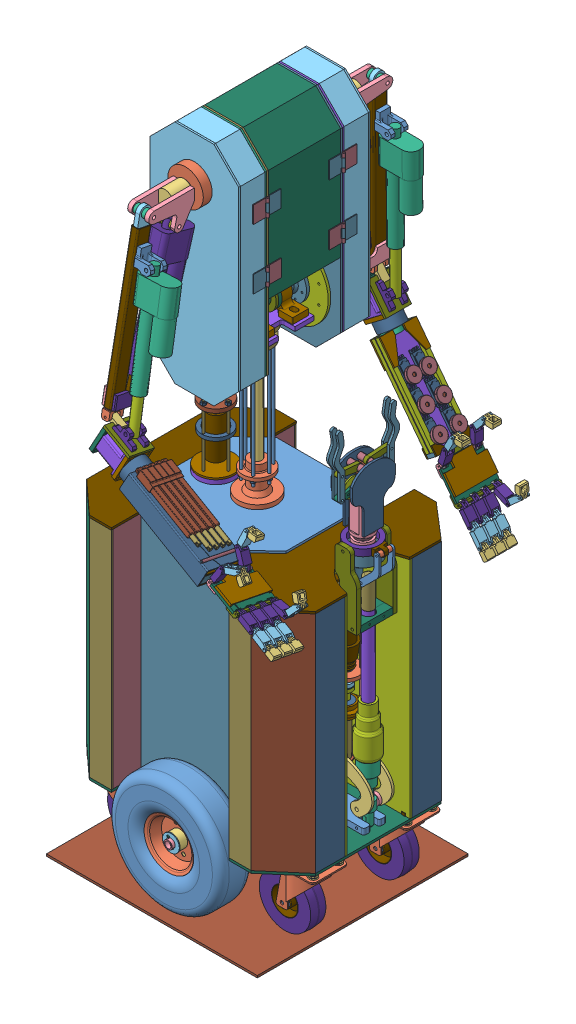
SolidWorks assembly sorbot, configuration По умолчанию. Lengths in mm. (continued)
Mates (geometry in assembly coordinates): (continued)
- Заблокировать432: lock: unknown of ?; unknown of ?
- Заблокировать433: lock: unknown of ?; unknown of ?
- Заблокировать434: lock: unknown of ?; unknown of ?
- Концентричный501: concentric aligned: cylinder of forearm.rotate-2/SY57STH56-2804A-1 through (17.8304 847.8969 -413.8911) axis (-0.604887 0.796311 0.000678) radius 3.175; cylinder of forearm.rotate.p2-2 through (17.165 848.7728 -413.8904) axis (-0.604887 0.796311 0.000678) radius 3.175
- Расстояние24: distance = 2 mm aligned: plane of forearm.rotate-2/forearm.rotate.p4-1 through (24.1212 839.6153 -413.8982) normal (0.604887 -0.796311 -0.000678); plane of forearm.rotate.p2-2 through (25.331 838.0226 -413.8995) normal (0.604887 -0.796311 -0.000678)
- Совпадение891: coincident anti-aligned: plane of forearm.rotate.p2-2 through (25.331 838.0226 -413.8995) normal (0.604887 -0.796311 -0.000678); plane of lower.arm.p1-2 through (36.5459 846.5524 -426.6459) normal (-0.604887 0.796311 0.000678)
- Заблокировать435: lock: unknown of ?; unknown of ?
- Заблокировать436: lock: unknown of ?; unknown of ?
- Заблокировать437: lock: unknown of ?; unknown of ?
- Заблокировать438: lock: unknown of ?; unknown of ?
- Заблокировать439: lock: unknown of ?; unknown of ?
- Заблокировать440: lock: unknown of ?; unknown of ?
- Заблокировать441: lock: unknown of ?; unknown of ?
- Заблокировать442: lock: unknown of ?; unknown of ?
- Заблокировать443: lock: unknown of ?; unknown of ?
- Заблокировать444: lock: unknown of ?; unknown of ?
- Заблокировать445: lock: unknown of ?; unknown of ?
- Параллельность201: parallel aligned: plane of forearm.rotate.p7-2 through (39.1177 879.8642 -383.6264) normal (0.796294 0.604869 0.00704); plane of lower.arm.p3-2 through (25.9039 838.4212 -370.8936) normal (0.796294 0.604869 0.00704)
- Заблокировать446: lock: unknown of ?; unknown of ?
- Заблокировать447: lock: unknown of ?; unknown of ?
- Заблокировать448: lock: unknown of ?; unknown of ?
- Заблокировать449: lock: unknown of ?; unknown of ?
- Заблокировать450: lock: unknown of ?; unknown of ?
- Заблокировать451: lock: unknown of ?; unknown of ?
- Концентричный504: concentric anti-aligned: cylinder of HS-311 Hitec Standard Servo and Horn-12/HS-311-p2-1 through (86.8297 780.9654 -431.4942) axis (0.796294 0.604869 0.00704) radius 4.064; cylinder of lower.arm.p9-8 through (91.8065 784.7458 -431.4502) axis (-0.796294 -0.604869 -0.00704) radius 12
- Концентричный505: concentric anti-aligned: cylinder of HS-311 Hitec Standard Servo and Horn-8/HS-311-p2-1 through (120.1178 737.1736 -434.1714) axis (0.796294 0.604869 0.00704) radius 4.064; cylinder of lower.arm.p9-10 through (125.0946 740.954 -434.1274) axis (-0.796294 -0.604869 -0.00704) radius 12
- Концентричный506: concentric anti-aligned: cylinder of HS-311 Hitec Standard Servo and Horn-10/HS-311-p2-1 through (153.4054 693.3815 -436.7686) axis (0.796294 0.604869 0.00704) radius 4.064; cylinder of lower.arm.p9-12 through (158.3823 697.1619 -436.7246) axis (-0.796294 -0.604869 -0.00704) radius 12
- Концентричный507: concentric anti-aligned: cylinder of HS-311 Hitec Standard Servo and Horn-11/HS-311-p2-1 through (86.6463 780.7961 -396.215) axis (0.796294 0.604869 0.00704) radius 4.064; cylinder of lower.arm.p9-7 through (91.6232 784.5765 -396.171) axis (-0.796294 -0.604869 -0.00704) radius 12
- Концентричный508: concentric anti-aligned: cylinder of HS-311 Hitec Standard Servo and Horn-7/HS-311-p2-1 through (119.907 736.979 -393.6124) axis (0.796294 0.604869 0.00704) radius 4.064; cylinder of lower.arm.p9-9 through (124.8838 740.7594 -393.5684) axis (-0.796294 -0.604869 -0.00704) radius 12
- Концентричный509: concentric anti-aligned: cylinder of HS-311 Hitec Standard Servo and Horn-9/HS-311-p2-1 through (153.1681 693.1623 -391.0897) axis (0.796294 0.604869 0.00704) radius 4.064; cylinder of lower.arm.p9-11 through (158.1449 696.9427 -391.0457) axis (-0.796294 -0.604869 -0.00704) radius 12
- Совпадение938: coincident anti-aligned: plane of HS-311 Hitec Standard Servo and Horn-12/HS-311-p2-1 through (93.1733 783.0442 -439.8505) normal (0.796294 0.604869 0.00704); plane of lower.arm.p9-8 through (91.8065 784.7458 -431.4502) normal (-0.796294 -0.604869 -0.00704)
- Совпадение939: coincident anti-aligned: plane of HS-311 Hitec Standard Servo and Horn-8/HS-311-p2-1 through (126.4614 739.2524 -442.5277) normal (0.796294 0.604869 0.00704); plane of lower.arm.p9-10 through (125.0946 740.954 -434.1274) normal (-0.796294 -0.604869 -0.00704)
- Совпадение940: coincident anti-aligned: plane of HS-311 Hitec Standard Servo and Horn-10/HS-311-p2-1 through (159.7491 695.4603 -445.1249) normal (0.796294 0.604869 0.00704); plane of lower.arm.p9-12 through (158.3823 697.1619 -436.7246) normal (-0.796294 -0.604869 -0.00704)
- Совпадение941: coincident anti-aligned: plane of HS-311 Hitec Standard Servo and Horn-9/HS-311-p2-1 through (159.5117 695.2411 -399.446) normal (0.796294 0.604869 0.00704); plane of lower.arm.p9-11 through (158.1449 696.9427 -391.0457) normal (-0.796294 -0.604869 -0.00704)
- Совпадение942: coincident anti-aligned: plane of HS-311 Hitec Standard Servo and Horn-7/HS-311-p2-1 through (126.2507 739.0578 -401.9687) normal (0.796294 0.604869 0.00704); plane of lower.arm.p9-9 through (124.8838 740.7594 -393.5684) normal (-0.796294 -0.604869 -0.00704)
- Совпадение943: coincident anti-aligned: plane of HS-311 Hitec Standard Servo and Horn-11/HS-311-p2-1 through (92.99 782.8749 -404.5714) normal (0.796294 0.604869 0.00704); plane of lower.arm.p9-7 through (91.6232 784.5765 -396.171) normal (-0.796294 -0.604869 -0.00704)
- Заблокировать452: lock: unknown of ?; unknown of ?
- Заблокировать453: lock: unknown of ?; unknown of ?
- Заблокировать454: lock: unknown of ?; unknown of ?
- Заблокировать455: lock: unknown of ?; unknown of ?
- Заблокировать456: lock: unknown of ?; unknown of ?
- Заблокировать457: lock: unknown of ?; unknown of ?
- Заблокировать458: lock: unknown of ?; unknown of ?
- Совпадение963: coincident anti-aligned: plane of palm.p1-4 through (227.4584 603.5642 -463.9754) normal (0.796294 0.604869 0.00704); plane of palm.p6-3 through (187.1247 655.9192 -400.1209) normal (-0.796294 -0.604869 -0.00704)
- Совпадение964: coincident anti-aligned: plane of palm.p1-4 through (227.4584 603.5642 -463.9754) normal (0.796294 0.604869 0.00704); plane of palm.p6-4 through (187.4607 655.8101 -428.7506) normal (-0.796294 -0.604869 -0.00704)
- Совпадение965: coincident anti-aligned: plane of palm.p1-4 through (227.4584 603.5642 -463.9754) normal (0.796294 0.604869 0.00704); plane of palm.p5-3 through (207.7743 628.5171 -381.4417) normal (-0.796294 -0.604869 -0.00704)
- Совпадение966: coincident anti-aligned: plane of palm.p1-4 through (227.4584 603.5642 -463.9754) normal (0.796294 0.604869 0.00704); plane of palm.p5-4 through (208.1815 628.7395 -446.6064) normal (-0.796294 -0.604869 -0.00704)
- Заблокировать459: lock: unknown of ?; unknown of ?
- Заблокировать460: lock: unknown of ?; unknown of ?
- Заблокировать461: lock: unknown of ?; unknown of ?
- Заблокировать462: lock: unknown of ?; unknown of ?
- Совпадение967: coincident anti-aligned: plane of palm.p1-4 through (227.4584 603.5642 -463.9754) normal (0.796294 0.604869 0.00704); plane of palm.cap-2 through (193.3919 648.1333 -440.0443) normal (-0.796294 -0.604869 -0.00704)
- Совпадение968: coincident aligned: plane of palm.p1-4 through (181.5722 662.8077 -363.9271) normal (-0.604887 0.796311 0.000678); plane of palm.cap-2 through (186.4741 666.5515 -387.7779) normal (-0.604887 0.796311 0.000678)
- Совпадение969: coincident aligned: plane of palm.p1-4 through (181.5722 662.8077 -363.9271) normal (-0.005196 -0.004798 0.999975); plane of palm.cap-2 through (224.3892 616.3597 -363.9275) normal (-0.005196 -0.004798 0.999975)
- Заблокировать463: lock: unknown of ?; unknown of ?
- Совпадение970: coincident anti-aligned: plane of palm.p1-4 through (222.6806 599.935 -464.0176) normal (-0.796294 -0.604869 -0.00704); plane of palm.p3.m-3 through (196.4062 633.3603 -363.9913) normal (0.796294 0.604869 0.00704)
- Совпадение971: coincident aligned: plane of palm.p1-4 through (181.5722 662.8077 -363.9271) normal (-0.005196 -0.004798 0.999975); plane of palm.p3.m-3 through (183.7598 663.2341 -363.9137) normal (-0.005196 -0.004798 0.999975)
- Совпадение972: coincident anti-aligned: plane of palm.p1-4 through (187.6419 654.8638 -367.9338) normal (-0.604887 0.796311 0.000678); plane of palm.p3.m-3 through (190.024 656.6699 -363.9126) normal (0.604887 -0.796311 -0.000678)
- Заблокировать464: lock: unknown of ?; unknown of ?
- Совпадение973: coincident anti-aligned: plane of palm.p1-4 through (222.6806 599.935 -464.0176) normal (-0.796294 -0.604869 -0.00704); plane of palm.p3.m-4 through (196.8141 633.737 -442.4893) normal (0.796294 0.604869 0.00704)
- Совпадение974: coincident aligned: plane of palm.p1-4 through (182.0918 663.2875 -463.9246) normal (0.005196 0.004798 -0.999975); plane of palm.p3.m-4 through (184.2795 663.7139 -463.9112) normal (0.005196 0.004798 -0.999975)
- Совпадение975: coincident anti-aligned: plane of palm.p1-4 through (188.1199 655.3052 -459.9315) normal (-0.604887 0.796311 0.000678); plane of palm.p3.m-4 through (190.4319 657.0465 -442.4107) normal (0.604887 -0.796311 -0.000678)
- Заблокировать465: lock: unknown of ?; unknown of ?
- Совпадение976: coincident anti-aligned: plane of palm.p1-4 through (222.6806 599.935 -464.0176) normal (-0.796294 -0.604869 -0.00704); plane of palm.p3-2 through (211.1232 615.1499 -464.0047) normal (0.796294 0.604869 0.00704)
- Совпадение977: coincident aligned: plane of palm.p1-4 through (181.5722 662.8077 -363.9271) normal (-0.005196 -0.004798 0.999975); plane of palm.p3-2 through (235.1796 598.0217 -363.9594) normal (-0.005196 -0.004798 0.999975)
- Совпадение978: coincident anti-aligned: plane of palm.p1-4 through (226.9387 603.0844 -363.9779) normal (0.604887 -0.796311 -0.000678); plane of palm.p3-2 through (230.2454 605.6812 -463.9508) normal (-0.604887 0.796311 0.000678)
- Заблокировать466: lock: unknown of ?; unknown of ?
- Концентричный510: concentric aligned: cylinder of palm.p3.m-3 through (183.124 657.0899 -363.9465) axis (0.005196 0.004798 -0.999975) radius 1.5; cylinder of finger.p1-7 through (183.1266 657.0923 -364.4464) axis (0.005196 0.004798 -0.999975) radius 1.5
- Совпадение979: coincident anti-aligned: plane of palm.p3.m-3 through (170.6462 660.8634 -381.4936) normal (-0.005196 -0.004798 0.999975); plane of finger.p1-7 through (175.0262 648.1576 -381.5318) normal (0.005196 0.004798 -0.999975)
- Концентричный512: concentric aligned: cylinder of finger.p2-13 through (195.1724 695.7619 -364.1983) axis (0.005196 0.004798 -0.999975) radius 1.5; cylinder of finger.p1-7 through (195.1724 695.7619 -364.1983) axis (0.005196 0.004798 -0.999975) radius 1.5
- Совпадение980: coincident anti-aligned: plane of finger.p1-7 through (188.6599 690.1 -380.7597) normal (-0.005196 -0.004798 0.999975); plane of finger.p2-13 through (186.283 688.6169 -380.7792) normal (0.005196 0.004798 -0.999975)
- Концентричный513: concentric aligned: cylinder of finger.p2-13 through (213.5888 730.1387 -363.9377) axis (0.005196 0.004798 -0.999975) radius 1.5; cylinder of finger.p3-7 through (213.5894 730.1393 -364.0505) axis (0.005196 0.004798 -0.999975) radius 1.5
- Совпадение981: coincident anti-aligned: plane of finger.p2-13 through (206.1663 725.732 -380.4978) normal (-0.005196 -0.004798 0.999975); plane of finger.p3-7 through (203.231 735.0842 -380.4682) normal (0.005196 0.004798 -0.999975)
- Заблокировать467: lock: unknown of ?; unknown of ?
- Заблокировать468: lock: unknown of ?; unknown of ?
- Заблокировать469: lock: unknown of ?; unknown of ?
- Концентричный514: concentric aligned: cylinder of palm.p3.m-4 through (183.532 657.4665 -442.4445) axis (0.005196 0.004798 -0.999975) radius 1.5; cylinder of finger.p1-8 through (183.5345 657.4689 -442.9445) axis (0.005196 0.004798 -0.999975) radius 1.5
- Совпадение982: coincident anti-aligned: plane of palm.p3.m-4 through (171.0542 661.24 -459.9917) normal (-0.005196 -0.004798 0.999975); plane of finger.p1-8 through (178.7439 646.3905 -460.023) normal (0.005196 0.004798 -0.999975)
- Концентричный515: concentric aligned: cylinder of finger.p1-8 through (182.5946 697.9606 -442.7551) axis (0.005196 0.004798 -0.999975) radius 1.5; cylinder of finger.p2-14 through (182.5946 697.9606 -442.7551) axis (0.005196 0.004798 -0.999975) radius 1.5
- Концентричный516: concentric aligned: cylinder of finger.p2-14 through (208.2525 727.3307 -442.4808) axis (0.005196 0.004798 -0.999975) radius 1.5; cylinder of finger.p3-8 through (208.2519 727.3302 -442.368) axis (0.005196 0.004798 -0.999975) radius 1.5
- Совпадение983: coincident anti-aligned: plane of finger.p2-14 through (199.9501 724.6624 -446.5369) normal (0.005196 0.004798 -0.999975); plane of finger.p3-8 through (197.8276 732.2116 -446.5117) normal (-0.005196 -0.004798 0.999975)
- Совпадение984: coincident anti-aligned: plane of finger.p1-8 through (178.2622 690.4916 -459.3138) normal (-0.005196 -0.004798 0.999975); plane of finger.p2-14 through (172.3135 693.0129 -459.3327) normal (0.005196 0.004798 -0.999975)
- Заблокировать470: lock: unknown of ?; unknown of ?
- Заблокировать471: lock: unknown of ?; unknown of ?
- Заблокировать472: lock: unknown of ?; unknown of ?
- Концентричный517: concentric aligned: cylinder of palm.p3-2 through (229.7871 599.6719 -463.982) axis (-0.005196 -0.004798 0.999975) radius 1.5; cylinder of ? through (229.3818 599.2976 -385.9839) axis (-0.005196 -0.004798 0.999975) radius 1.5
- Совпадение985: coincident anti-aligned: plane of palm.p3-2 through (217.197 599.4357 -369.0462) normal (0.005196 0.004798 -0.999975); plane of ? through (218.5938 605.036 -369.012) normal (-0.005196 -0.004798 0.999975)
- Заблокировать473: lock: unknown of ?
- Концентричный518: concentric aligned: cylinder of ? through (253.4816 566.7446 -386.0149) axis (-0.005196 -0.004798 0.999975) radius 1.5; cylinder of ? through (253.4816 566.7446 -386.0149) axis (-0.005196 -0.004798 0.999975) radius 1.5
- Совпадение986: coincident anti-aligned: plane of ? through (245.2759 569.9159 -369.5419) normal (0.005196 0.004798 -0.999975); plane of ? through (243.3968 572.3896 -369.5398) normal (-0.005196 -0.004798 0.999975)
- Заблокировать474: lock: unknown of ?; unknown of ?
- Концентричный519: concentric aligned: cylinder of ? through (277.0722 535.6885 -386.0413) axis (-0.005196 -0.004798 0.999975) radius 1.5; cylinder of ? through (277.0716 535.6879 -385.9285) axis (-0.005196 -0.004798 0.999975) radius 1.5
- Совпадение987: coincident anti-aligned: plane of ? through (268.8665 538.8597 -369.5683) normal (0.005196 0.004798 -0.999975); plane of ? through (266.9874 541.3335 -369.5662) normal (-0.005196 -0.004798 0.999975)
- Заблокировать475: lock: unknown of ?; unknown of ?
- Концентричный520: concentric aligned: cylinder of palm.p3-2 through (229.7871 599.6719 -463.982) axis (-0.005196 -0.004798 0.999975) radius 1.5; cylinder of finger.p1-10 through (229.5143 599.42 -411.4833) axis (-0.005196 -0.004798 0.999975) radius 1.5
- Совпадение988: coincident anti-aligned: plane of palm.p3-2 through (224.5881 590.0023 -394.5537) normal (0.005196 0.004798 -0.999975); plane of finger.p1-10 through (218.7263 605.1583 -394.5114) normal (-0.005196 -0.004798 0.999975)
- Заблокировать476: lock: unknown of ?; unknown of ?
- Концентричный521: concentric aligned: cylinder of finger.p1-10 through (253.6141 566.867 -411.5143) axis (-0.005196 -0.004798 0.999975) radius 1.5; cylinder of finger.p2-16 through (253.6141 566.867 -411.5143) axis (-0.005196 -0.004798 0.999975) radius 1.5
- Совпадение989: coincident anti-aligned: plane of finger.p1-10 through (245.4084 570.0382 -395.0413) normal (0.005196 0.004798 -0.999975); plane of finger.p2-16 through (243.5293 572.512 -395.0392) normal (-0.005196 -0.004798 0.999975)
- Заблокировать477: lock: unknown of ?; unknown of ?
- Концентричный522: concentric aligned: cylinder of finger.p2-16 through (277.2047 535.8108 -411.5407) axis (-0.005196 -0.004798 0.999975) radius 1.5; cylinder of finger.p3-10 through (277.2041 535.8103 -411.4278) axis (-0.005196 -0.004798 0.999975) radius 1.5
- Совпадение990: coincident anti-aligned: plane of finger.p2-16 through (268.999 538.9821 -395.0677) normal (0.005196 0.004798 -0.999975); plane of finger.p3-10 through (267.1199 541.4559 -395.0656) normal (-0.005196 -0.004798 0.999975)
- Заблокировать478: lock: unknown of ?; unknown of ?
- Концентричный523: concentric aligned: cylinder of palm.p3-2 through (229.7871 599.6719 -463.982) axis (-0.005196 -0.004798 0.999975) radius 1.5; cylinder of finger.p1-11 through (229.6468 599.5423 -436.9827) axis (-0.005196 -0.004798 0.999975) radius 1.5
- Совпадение991: coincident anti-aligned: plane of palm.p3-2 through (224.7206 590.1246 -420.053) normal (0.005196 0.004798 -0.999975); plane of finger.p1-11 through (218.8588 605.2807 -420.0108) normal (-0.005196 -0.004798 0.999975)
- Заблокировать479: lock: unknown of ?; unknown of ?
- Концентричный524: concentric aligned: cylinder of finger.p1-11 through (253.7466 566.9893 -437.0136) axis (-0.005196 -0.004798 0.999975) radius 1.5; cylinder of finger.p2-17 through (253.7466 566.9893 -437.0136) axis (-0.005196 -0.004798 0.999975) radius 1.5
- Совпадение992: coincident anti-aligned: plane of finger.p1-11 through (245.5409 570.1606 -420.5406) normal (0.005196 0.004798 -0.999975); plane of finger.p2-17 through (243.6618 572.6343 -420.5385) normal (-0.005196 -0.004798 0.999975)
- Заблокировать480: lock: unknown of ?; unknown of ?
- Концентричный525: concentric aligned: cylinder of finger.p2-17 through (277.3372 535.9332 -437.04) axis (-0.005196 -0.004798 0.999975) radius 1.5; cylinder of finger.p3-11 through (277.3366 535.9327 -436.9272) axis (-0.005196 -0.004798 0.999975) radius 1.5
- Совпадение993: coincident anti-aligned: plane of finger.p2-17 through (269.1315 539.1044 -420.5671) normal (0.005196 0.004798 -0.999975); plane of finger.p3-11 through (267.2524 541.5782 -420.565) normal (-0.005196 -0.004798 0.999975)
- Заблокировать481: lock: unknown of ?; unknown of ?
- Концентричный526: concentric aligned: cylinder of palm.p3-2 through (229.7871 599.6719 -463.982) axis (-0.005196 -0.004798 0.999975) radius 1.5; cylinder of finger.p1-12 through (229.7793 599.6647 -462.482) axis (-0.005196 -0.004798 0.999975) radius 1.5
- Совпадение994: coincident anti-aligned: plane of palm.p3-2 through (217.5945 599.8027 -445.5442) normal (0.005196 0.004798 -0.999975); plane of finger.p1-12 through (217.5121 599.4267 -445.5465) normal (-0.005196 -0.004798 0.999975)
- Концентричный527: concentric aligned: cylinder of finger.p1-12 through (266.7206 583.0564 -462.3697) axis (-0.005196 -0.004798 0.999975) radius 1.5; cylinder of finger.p2-18 through (266.7206 583.0564 -462.3697) axis (-0.005196 -0.004798 0.999975) radius 1.5
- Совпадение995: coincident anti-aligned: plane of finger.p1-12 through (257.9626 581.8413 -445.9207) normal (0.005196 0.004798 -0.999975); plane of finger.p2-18 through (261.791 572.5236 -445.9455) normal (-0.005196 -0.004798 0.999975)
- Концентричный528: concentric aligned: cylinder of finger.p2-18 through (295.6349 609.2268 -462.0939) axis (-0.005196 -0.004798 0.999975) radius 1.5; cylinder of finger.p3-12 through (295.6343 609.2262 -461.9811) axis (-0.005196 -0.004798 0.999975) radius 1.5
- Совпадение996: coincident anti-aligned: plane of finger.p2-18 through (293.0084 600.7785 -445.6477) normal (0.005196 0.004798 -0.999975); plane of finger.p3-12 through (300.8404 598.9128 -445.6159) normal (-0.005196 -0.004798 0.999975)
- Заблокировать482: lock: unknown of ?; unknown of ?
- Заблокировать483: lock: unknown of ?; unknown of ?
- Заблокировать484: lock: unknown of ?; unknown of ?
- Заблокировать485: lock: unknown of ?; unknown of ?
- Концентричный529: concentric aligned: cylinder of body_axis-1 through (-20.0648 1016.5246 -50.7475) axis (0 0 -1) radius 9; cylinder of bodu.tilit.axis.enforcement-1 through (-20.0648 1016.5246 -50.7475) axis (0 0 -1) radius 9
- Совпадение999: coincident aligned: plane of body_axis-1 through (-20.0648 1016.5246 -221.0975) normal (0 0 -1); plane of bodu.tilit.axis.enforcement-1 through (-20.0648 1016.5246 -221.0975) normal (0 0 -1)
- Заблокировать486: lock: unknown of ?; unknown of ?
- Заблокировать488: lock: unknown of turret.table-1; unknown of ?
- Заблокировать489: lock: unknown of turret.table-1; unknown of ?
- Заблокировать490: lock: unknown of turret.table-1; unknown of ?
- Заблокировать491: lock: unknown of turret.table-1; unknown of ?
- Заблокировать492: lock: unknown of turret.table-1; unknown of ?
- Заблокировать493: lock: unknown of turret.table-1; unknown of ?
- Совпадение1001: coincident anti-aligned: plane of m6.nut-1 through (8.0892 944.0246 -131.6914) normal (0 -1 0); plane of body_pivot_fixture-1 through (-20.0648 944.0246 -136.9555) normal (0 1 0)
- Концентричный530: concentric aligned: cylinder of ? through (8.0892 955.7352 -137.4649) axis (0 -1 0) radius 3; cylinder of m6.nut-1 through (8.0892 949.5246 -137.4649) axis (0 -1 0) radius 3
- Совпадение1002: coincident anti-aligned: plane of m6.nut-2 through (-6.429 944.0246 -155.8188) normal (0 -1 0); plane of body_pivot_fixture-1 through (-20.0648 944.0246 -136.9555) normal (0 1 0)
- Концентричный531: concentric aligned: cylinder of ? through (-6.429 955.7352 -161.5923) axis (0 -1 0) radius 3; cylinder of m6.nut-2 through (-6.429 949.5246 -161.5923) axis (0 -1 0) radius 3
- Совпадение1004: coincident anti-aligned: plane of m6.nut-3 through (-48.2188 944.0246 -130.6725) normal (0 -1 0); plane of body_pivot_fixture-1 through (-20.0648 944.0246 -136.9555) normal (0 1 0)
- Совпадение1005: coincident anti-aligned: plane of m6.nut-4 through (-34.583 944.0246 -155.3093) normal (0 -1 0); plane of body_pivot_fixture-1 through (-20.0648 944.0246 -136.9555) normal (0 1 0)
- Совпадение1006: coincident anti-aligned: plane of m6.nut-5 through (-5.5466 944.0246 -107.0546) normal (0 -1 0); plane of body_pivot_fixture-1 through (-20.0648 944.0246 -136.9555) normal (0 1 0)
- Совпадение1007: coincident anti-aligned: plane of m6.nut-6 through (-33.7006 944.0246 -106.5452) normal (0 -1 0); plane of body_pivot_fixture-1 through (-20.0648 944.0246 -136.9555) normal (0 1 0)
- Концентричный532: concentric aligned: cylinder of ? through (-48.2188 955.7352 -136.446) axis (0 -1 0) radius 3; cylinder of m6.nut-3 through (-48.2188 949.5246 -136.446) axis (0 -1 0) radius 3
- Концентричный533: concentric aligned: cylinder of ? through (-34.583 955.7352 -161.0828) axis (0 -1 0) radius 3; cylinder of m6.nut-4 through (-34.583 949.5246 -161.0828) axis (0 -1 0) radius 3
- Концентричный534: concentric aligned: cylinder of ? through (-5.5466 955.7352 -112.8281) axis (0 -1 0) radius 3; cylinder of m6.nut-5 through (-5.5466 949.5246 -112.8281) axis (0 -1 0) radius 3
- Концентричный535: concentric aligned: cylinder of ? through (-33.7006 955.7352 -112.3187) axis (0 -1 0) radius 3; cylinder of m6.nut-6 through (-33.7006 949.5246 -112.3187) axis (0 -1 0) radius 3
- Совпадение1008: coincident anti-aligned: plane of ? through (-20.0648 662.7934 -136.9555) normal (0 -1 0); plane of m6.nut-12 through (-48.2188 662.7934 -130.6725) normal (0 1 0)
- Концентричный536: concentric aligned: cylinder of ? through (-48.2188 955.7352 -136.446) axis (0 -1 0) radius 3; cylinder of m6.nut-12 through (-48.2188 662.7934 -136.446) axis (0 -1 0) radius 3
- Совпадение1009: coincident anti-aligned: plane of ? through (-20.0648 662.7934 -136.9555) normal (0 -1 0); plane of m6.nut-11 through (-33.7006 662.7934 -106.5452) normal (0 1 0)
- Концентричный537: concentric aligned: cylinder of ? through (-33.7006 955.7352 -112.3187) axis (0 -1 0) radius 3; cylinder of m6.nut-11 through (-33.7006 662.7934 -112.3187) axis (0 -1 0) radius 3
- Совпадение1010: coincident anti-aligned: plane of ? through (-20.0648 662.7934 -136.9555) normal (0 -1 0); plane of m6.nut-7 through (-5.5466 662.7934 -107.0546) normal (0 1 0)
- Концентричный538: concentric aligned: cylinder of ? through (-5.5466 955.7352 -112.8281) axis (0 -1 0) radius 3; cylinder of m6.nut-7 through (-5.5466 662.7934 -112.8281) axis (0 -1 0) radius 3
- Совпадение1011: coincident anti-aligned: plane of ? through (-20.0648 662.7934 -136.9555) normal (0 -1 0); plane of m6.nut-8 through (-34.583 662.7934 -155.3093) normal (0 1 0)
- Концентричный539: concentric aligned: cylinder of ? through (-34.583 955.7352 -161.0828) axis (0 -1 0) radius 3; cylinder of m6.nut-8 through (-34.583 662.7934 -161.0828) axis (0 -1 0) radius 3
- Совпадение1012: coincident anti-aligned: plane of ? through (-20.0648 662.7934 -136.9555) normal (0 -1 0); plane of m6.nut-10 through (-6.429 662.7934 -155.8188) normal (0 1 0)
- Концентричный540: concentric aligned: cylinder of ? through (-6.429 955.7352 -161.5923) axis (0 -1 0) radius 3; cylinder of m6.nut-10 through (-6.429 662.7934 -161.5923) axis (0 -1 0) radius 3
- Совпадение1013: coincident anti-aligned: plane of ? through (-20.0648 662.7934 -136.9555) normal (0 -1 0); plane of m6.nut-9 through (8.0892 662.7934 -131.6914) normal (0 1 0)
- Концентричный541: concentric aligned: cylinder of ? through (8.0892 955.7352 -137.4649) axis (0 -1 0) radius 3; cylinder of m6.nut-9 through (8.0892 662.7934 -137.4649) axis (0 -1 0) radius 3
- Концентричный542: concentric anti-aligned: cylinder of body_tilt_lever_axis-1 through (-99.3474 976.856 -80.4875) axis (0 0 -1) radius 5; cylinder of body.tilt.intermediate.enforce-1 through (-99.3474 976.856 -149.5942) axis (0 0 1) radius 5
- Совпадение1014: coincident anti-aligned: plane of body_tilt_lever-2 through (-97.2168 978.7734 -124.5942) normal (0 0 -1); plane of body.tilt.intermediate.enforce-1 through (-99.3474 976.856 -124.5942) normal (0 0 1)
- Заблокировать498: lock: unknown of arm.fixture.cap-2; unknown of body.frame.p1-left-1
- Заблокировать499: lock: unknown of body.tilit.enforcement-2; unknown of body.frame.p1-left-1
- Заблокировать500: lock: unknown of body.frame.p2-1; unknown of body.frame.p1-left-1
- Заблокировать501: lock: unknown of body_tilt_drive_frame_cap-1; unknown of body.frame.p3-1
- Совпадение1021: coincident anti-aligned: plane of body.frame.p1-left-1 through (92.5148 1436.2936 -222.3595) normal (0 0 1); plane of arm.drive.motor.pair-1 through (3.7745 1243.7974 -222.3595) normal (0 0 -1)
- Совпадение1022: coincident anti-aligned: plane of body.frame.p1-3 through (92.5097 1436.2936 -50.7442) normal (0 0 -1); plane of arm.drive.motor-1 through (-20.8275 1162.0905 -50.7442) normal (0 0 1)
- Концентричный546: concentric aligned: cylinder of forearm.rotate.p12-m-2 through (-28.3182 975.8779 -381.2699) axis (0.999986 0 0.005196) radius 4; cylinder of arm.actuator.p2-5 through (-37.3181 975.8779 -381.3167) axis (0.999986 0 0.005196) radius 4
- Концентричный547: concentric anti-aligned: cylinder of arm.actuator.p2-5 through (-12.3145 967.4115 -381.9422) axis (-0.000462 0.996043 0.088876) radius 10; cylinder of arm.actuator-5/arm.actuator.p1-1 through (-12.4006 1153.2182 -365.3628) axis (0.000462 -0.996043 -0.088876) radius 10
- Концентричный549: concentric anti-aligned: cylinder of arm.drive.p3-1 through (3.7745 1243.7974 -65.7442) axis (0 0 1) radius 6; cylinder of arm.drive.p5-1 through (3.7745 1243.7974 -50.7442) axis (0 0 -1) radius 6
- Совпадение1023: coincident anti-aligned: plane of body.frame.p1-3 through (92.5097 1436.2936 -50.7442) normal (0 0 -1); plane of arm.drive.p5-1 through (3.7745 1243.7974 -50.7442) normal (0 0 1)
- Концентричный550: concentric anti-aligned: cylinder of arm.drive.p3-1 through (3.7745 1243.7974 -65.7442) axis (0 0 1) radius 6; cylinder of arm.drive.p6-1 through (3.7745 1243.7974 -50.7442) axis (0 0 -1) radius 7
- Совпадение1024: coincident anti-aligned: plane of body.frame.p1-3 through (92.5097 1436.2936 -50.7442) normal (0 0 -1); plane of arm.drive.p6-1 through (3.7745 1243.7974 -50.7442) normal (0 0 1)
- Концентричный551: concentric anti-aligned: cylinder of arm.drive.p3-1 through (3.7745 1243.7974 -65.7442) axis (0 0 1) radius 6; cylinder of arm.drive.motor.pair-1 through (3.7745 1243.7974 -192.8595) axis (0 0 -1) radius 8
- Заблокировать504: lock: unknown of body.frame.p1-left-1; unknown of arm.drive.motor.pair-1
- Совпадение1028: coincident anti-aligned: plane of body.frame.p1-left-1 through (92.5148 1436.2936 -222.3595) normal (0 0 1); plane of arm.drive.p3-2 through (-20.8275 1162.0905 -222.3595) normal (0 0 -1)
- Концентричный553: concentric anti-aligned: cylinder of arm.drive.motor-1 through (-20.8275 1162.0905 -80.2442) axis (0 0 1) radius 8; cylinder of arm.drive.p3-2 through (-20.8275 1162.0905 -207.3595) axis (0 0 -1) radius 6
- Концентричный554: concentric anti-aligned: cylinder of arm.drive.p3-2 through (-20.8275 1162.0905 -207.3595) axis (0 0 -1) radius 6; cylinder of arm.drive.p5-2 through (-20.8275 1162.0905 -222.3595) axis (0 0 1) radius 6
- Совпадение1029: coincident anti-aligned: plane of body.frame.p1-left-1 through (92.5148 1436.2936 -222.3595) normal (0 0 1); plane of arm.drive.p5-2 through (-20.8275 1162.0905 -222.3595) normal (0 0 -1)
- Совпадение1030: coincident anti-aligned: plane of body.frame.p1-left-1 through (92.5148 1436.2936 -222.3595) normal (0 0 1); plane of arm.drive.p6-2 through (-20.8275 1162.0905 -222.3595) normal (0 0 -1)
- Концентричный555: concentric anti-aligned: cylinder of arm.drive.p3-2 through (-20.8275 1162.0905 -207.3595) axis (0 0 -1) radius 6; cylinder of arm.drive.p6-2 through (-20.8275 1162.0905 -222.3595) axis (0 0 1) radius 7
- Заблокировать505: lock: unknown of body.frame.p1-3; unknown of ?
- Заблокировать506: lock: unknown of body.frame.p1-left-1; unknown of ?
- Заблокировать507: lock: unknown of body.frame.p1-3; unknown of ?
- Заблокировать508: lock: unknown of body.frame.p1-3; unknown of arm.drive.p6-1
- Заблокировать510: lock: unknown of ?; unknown of ?
- Концентричный559: concentric anti-aligned: cylinder of arm.drive.p3-2 through (-20.8275 1162.0905 -207.3595) axis (0 0 -1) radius 6; cylinder of m14.nut-1 through (-20.8275 1162.0905 -128.9852) axis (0 0 1) radius 7
- Совпадение1034: coincident anti-aligned: plane of arm.drive.p7-2 through (-42.4721 1162.0905 -109.4852) normal (0 1 0); plane of arm.drive.p7-3 through (-42.4721 1162.0905 -137.4852) normal (0 -1 0)
- Совпадение1035: coincident aligned: plane of arm.drive.p7-2 through (12.3724 1162.0905 -109.4852) normal (0 0 1); plane of arm.drive.p7-3 through (12.3724 1162.0905 -109.4852) normal (0 0 1)
- Совпадение1036: coincident aligned: plane of arm.drive.p7-2 through (-42.4721 1162.0905 -137.4852) normal (-1 0 0); plane of arm.drive.p7-3 through (-42.4721 1162.0905 -109.4852) normal (-1 0 0)
- Концентричный560: concentric anti-aligned: cylinder of ? through (10.8018 1164.5905 -123.4852) axis (0 -1 0) radius 2.5; cylinder of arm.drive.p7-3 through (10.8018 1162.0905 -123.4852) axis (0 1 0) radius 2.5
- Совпадение1038: coincident anti-aligned: plane of m14.nut-1 through (-8.1258 1162.0905 -128.9852) normal (0 0 -1); plane of arm.drive.p7-3 through (-33.7738 1162.0905 -128.9852) normal (0 0 1)
- Заблокировать511: lock: unknown of ?; unknown of ?
- Совпадение1040: coincident anti-aligned: plane of arm.drive.p7-4 through (-9.0342 1232.7974 -150.3) normal (0 1 0); plane of m14.nut-2 through (-2.5764 1232.7974 -139.8) normal (0 -1 0)
- Совпадение1041: coincident anti-aligned: plane of m14.nut-2 through (-2.5764 1254.7974 -150.3) normal (0 0 -1); plane of arm.drive.p7-4 through (-9.0341 1243.9206 -150.3) normal (0 0 1)
- Совпадение1042: coincident: plane of arm.drive.p7-4 through (16.4762 1232.7974 -150.3) normal (-1 0 0); line of m14.nut-2 through (16.4762 1243.7974 -140.8) axis (0 0 -1)
- Заблокировать512: lock: unknown of ?; unknown of ?
- Концентричный562: concentric anti-aligned: cylinder of m14.nut-2 through (3.7745 1243.7974 -139.8) axis (0 0 -1) radius 7; cylinder of arm.drive.p3-1 through (3.7745 1243.7974 -65.7442) axis (0 0 1) radius 6
- Совпадение1043: coincident anti-aligned: plane of arm.drive.p7-5 through (-17.7325 1243.9206 -159.3) normal (0 -1 0); plane of arm.drive.p7-4 through (-17.7325 1243.9206 -131.3) normal (0 1 0)
- Концентричный563: concentric anti-aligned: cylinder of arm.drive.p7-4 through (35.5414 1243.9206 -145.3) axis (0 -1 0) radius 2.5; cylinder of arm.drive.p7-5 through (35.5414 1243.9206 -145.3) axis (0 1 0) radius 2.5
- Совпадение1045: coincident aligned: plane of arm.drive.p7-4 through (-17.7325 1243.9206 -159.3) normal (-1 0 0); plane of arm.drive.p7-5 through (-17.7325 1243.9206 -131.3) normal (-1 0 0)
- Совпадение1046: coincident aligned: plane of arm.drive.p7-4 through (37.112 1243.9206 -131.3) normal (0 0 1); plane of arm.drive.p7-5 through (37.112 1243.9206 -131.3) normal (0 0 1)
- Концентричный564: concentric anti-aligned: cylinder of ? through (35.5414 1246.2974 -145.3) axis (0 -1 0) radius 2.5; cylinder of arm.drive.p7-5 through (35.5414 1243.9206 -145.3) axis (0 1 0) radius 2.5
- Совпадение1047: coincident anti-aligned: plane of body.frame.p4-4 through (-117.3772 1436.2936 -230.3595) normal (0 0 -1); plane of arm.drive.p1.m1-1 through (28.6519 1174.5905 -230.3595) normal (0 0 1)
- Совпадение1048: coincident anti-aligned: plane of body.frame.p4-4 through (-117.3772 1436.2936 -230.3595) normal (0 0 -1); plane of arm.drive.p1.m1-2 through (28.6519 1159.5905 -230.3595) normal (0 0 1)
- Параллельность203: parallel anti-aligned: plane of arm.drive.p1.m1-1 through (28.6519 1164.5905 -234.3595) normal (0 -1 0); plane of arm.drive.p1.m1-2 through (28.6519 1159.5905 -234.3595) normal (0 1 0)
- Совпадение1051: coincident anti-aligned: plane of ? through (48.6519 1164.5905 -237.3595) normal (0 1 0); plane of arm.drive.p1.m1-1 through (28.6519 1164.5905 -234.3595) normal (0 -1 0)
- Совпадение1052: coincident aligned: plane of arm.drive.p1.m1-1 through (68.6519 1174.5904 -230.3595) normal (1 0 0); plane of arm.drive.p1.m1-2 through (68.6519 1159.5904 -230.3595) normal (1 0 0)
- Совпадение1053: coincident anti-aligned: plane of ? through (48.6519 1159.5905 -237.3595) normal (0 -1 0); plane of arm.drive.p1.m1-2 through (28.6519 1159.5905 -234.3595) normal (0 1 0)
- Заблокировать513: lock: unknown of ?; unknown of ?
- Заблокировать514: lock: unknown of ?; unknown of ?
- Концентричный565: concentric aligned: cylinder of ? through (48.6519 1164.5905 -237.3595) axis (0 -1 0) radius 2.5; cylinder of arm.drive.p1.m1-2 through (48.6519 1159.5905 -237.3595) axis (0 -1 0) radius 2.5
- Концентричный566: concentric anti-aligned: cylinder of shoulder.bearing.housing-3 through (-12.6499 1335.3853 -313.3595) axis (0 0 1) radius 15.5; cylinder of body.frame.p4.external-1 through (-12.6499 1335.3853 -288.3595) axis (0 0 -1) radius 21
- Заблокировать516: lock: unknown of ?; unknown of ?
- Заблокировать517: lock: unknown of ?; unknown of ?
- Заблокировать518: lock: unknown of ?; unknown of ?
- Концентричный567: concentric aligned: cylinder of shoulder.bearing.housing-1 through (-12.7629 1335.3853 40.2558) axis (0 0 -1) radius 15.5; cylinder of body.frame.p4.external-2 through (-12.7629 1335.3853 19.2558) axis (0 0 -1) radius 21
- Заблокировать520: lock: unknown of body.frame.p5-1; unknown of body.frame.p4.external-2
- Заблокировать522: lock: unknown of arm.lift.actuator.fixture.p3-1; unknown of body.frame.p4.external-2
- Заблокировать523: lock: unknown of shoulder.bearing.housing-1; unknown of body.frame.p4.external-2
- Заблокировать524: lock: unknown of arm.lift.actuator.fixture.p2-1; unknown of arm.lift.actuator.fixture.p3-1
- Совпадение1061: coincident anti-aligned: plane of ? through (45.4163 1246.2974 -35.7442) normal (0 1 0); plane of arm.drive.p1.m1-4 through (65.4163 1246.2974 -38.7442) normal (0 -1 0)
- Совпадение1064: coincident aligned: plane of arm.drive.p1.m1-3 through (65.4163 1241.2974 -42.7442) normal (1 0 0); plane of arm.drive.p1.m1-4 through (65.4163 1256.2974 -42.7442) normal (1 0 0)
- Совпадение1065: coincident anti-aligned: plane of ? through (45.4163 1241.2974 -35.7442) normal (0 -1 0); plane of arm.drive.p1.m1-3 through (65.4163 1241.2974 -38.7442) normal (0 1 0)
- Концентричный568: concentric aligned: cylinder of ? through (45.4163 1246.2974 -35.7442) axis (0 -1 0) radius 2.5; cylinder of arm.drive.p1.m1-4 through (45.4163 1256.2974 -35.7442) axis (0 -1 0) radius 2.5
- Концентричный569: concentric anti-aligned: cylinder of shoulder.bearing.housing-2 through (-12.4903 1335.516 -67.7442) axis (0 0 1) radius 15.5; cylinder of body.frame.p4.right-1 through (-12.4903 1335.516 -42.7442) axis (0 0 -1) radius 12.5
- Заблокировать527: lock: unknown of arm.lift.actuator.fixture.p3-2; unknown of body.frame.p4.right-1
- Заблокировать528: lock: unknown of shoulder.bearing.housing-2; unknown of body.frame.p4.right-1
- Заблокировать529: lock: unknown of body.frame.p5-1; unknown of body.frame.p4.right-1
- Заблокировать530: lock: unknown of arm.drive.p1.m1-4; unknown of body.frame.p4.right-1
- Заблокировать531: lock: unknown of arm.drive.p1.m1-3; unknown of body.frame.p4.right-1
- Совпадение1067: coincident anti-aligned: plane of body.frame.p1-3 through (92.5097 1436.2936 -46.7442) normal (0 0 1); plane of body.frame.p4.right-1 through (-117.4903 1436.2936 -46.7442) normal (0 0 -1)
- Совпадение1026: coincident anti-aligned: plane of body.frame.p4-4 through (-117.3772 1436.2936 -226.3595) normal (0 0 1); plane of body.frame.p1-left-1 through (92.5148 1436.2936 -226.3595) normal (0 0 -1)
- Концентричный570: concentric aligned: cylinder of arm.drive.motor-1 through (-20.8275 1162.0905 -80.2442) axis (0 0 1) radius 8; cylinder of arm.drive.p8-1 through (-20.8275 1162.0905 -80.2442) axis (0 0 1) radius 8
- Совпадение1069: coincident anti-aligned: plane of arm.drive.motor-1 through (-20.8275 1162.0905 -72.7442) normal (0 0 -1); plane of arm.drive.p8-1 through (-20.8275 1162.0905 -72.7442) normal (0 0 1)
- Концентричный571: concentric aligned: cylinder of arm.drive.motor.pair-1 through (3.7745 1243.7974 -192.8595) axis (0 0 -1) radius 8; cylinder of arm.drive.p8-2 through (3.7745 1243.7974 -192.8595) axis (0 0 -1) radius 8
- Совпадение1070: coincident anti-aligned: plane of arm.drive.motor.pair-1 through (3.7745 1243.7974 -200.3595) normal (0 0 1); plane of arm.drive.p8-2 through (3.7745 1243.7974 -200.3595) normal (0 0 -1)
- Концентричный572: concentric aligned: cylinder of man1.drive1-1 through (-118.5699 773.978 -137.5376) axis (0 -1 0) radius 6; cylinder of tilt.thread.rod.fixture.2-1 through (-118.5699 819.5591 -137.5376) axis (0 -1 0) radius 12
- Совпадение1071: coincident anti-aligned: plane of turret.table-1 through (-21.0698 612.7934 -363.9712) normal (0 1 0); plane of body.tilit.planetary.drive.fixture.p1-1 through (-118.5699 612.7934 -137.5376) normal (0 -1 0)
- Концентричный573: concentric aligned: cylinder of man1.drive1-1 through (-118.5699 703.728 -137.5376) axis (0 -1 0) radius 19; cylinder of body.tilit.planetary.drive.fixture.p1-1 through (-118.5699 622.7934 -137.5376) axis (0 -1 0) radius 42.5
- Заблокировать532: lock: unknown of turret.table-1; unknown of body.tilit.planetary.drive.fixture.p1-1
- Совпадение1072: coincident anti-aligned: plane of body.tilit.planetary.drive.fixture.p1-1 through (-118.5699 622.7934 -137.5376) normal (0 1 0); plane of body.tilit.planetary.drive.fixture.p2-1 through (-118.5699 622.7934 -137.5376) normal (0 -1 0)
- Концентричный575: concentric aligned: cylinder of body.tilit.planetary.drive.fixture.p1-1 through (-118.5699 622.7934 -137.5376) axis (0 -1 0) radius 42.5; cylinder of body.tilit.planetary.drive.fixture.p2-1 through (-118.5699 626.7934 -137.5376) axis (0 -1 0) radius 42.5
- Концентричный577: concentric aligned: cylinder of man1.drive1-1 through (-118.5699 773.978 -137.5376) axis (0 -1 0) radius 6; cylinder of tilt.thread.rod.fixture.2-2 through (-118.5699 792.5591 -137.5376) axis (0 -1 0) radius 8
- Совпадение1073: coincident anti-aligned: plane of tilt.thread.rod.fixture.2-1 through (-118.5699 793.5591 -137.5376) normal (0 -1 0); plane of tilt.thread.rod.fixture.2-2 through (-118.5699 793.5591 -137.5376) normal (0 1 0)
- Концентричный578: concentric aligned: cylinder of man1.drive1-1 through (-118.5699 703.728 -137.5376) axis (0 -1 0) radius 19; cylinder of body.tilit.planetary.drive.fixture.p3-1 through (-118.5699 703.728 -137.5376) axis (0 -1 0) radius 19
- Совпадение1074: coincident anti-aligned: plane of man1.drive1-1 through (-118.5699 703.728 -137.5376) normal (0 -1 0); plane of body.tilit.planetary.drive.fixture.p3-1 through (-118.5699 703.728 -137.5376) normal (0 1 0)
- Концентричный579: concentric aligned: cylinder of man1.drive1-1 through (-118.5699 761.728 -137.5376) axis (0 -1 0) radius 14.75; cylinder of body.tilit.planetary.drive.fixture.p4-1 through (-118.5699 762.9526 -137.5376) axis (0 -1 0) radius 14.8
- Заблокировать533: lock: unknown of man1.drive1-1; unknown of body.tilit.planetary.drive.fixture.p4-1
- Концентричный580: concentric anti-aligned: cylinder of body.tilit.planetary.drive.fixture.p3-1 through (-148.0595 695.728 -137.5376) axis (0 1 0) radius 2.5; cylinder of body.tilit.planetary.drive.fixture.p5-1 through (-148.0595 769.7934 -137.5376) axis (0 -1 0) radius 2.5
- Совпадение1076: coincident aligned: plane of body.tilit.planetary.drive.fixture.p1-1 through (-118.5699 612.7934 -137.5376) normal (0 -1 0); plane of body.tilit.planetary.drive.fixture.p5-1 through (-148.0595 612.7934 -137.5376) normal (0 -1 0)
- Совпадение1077: coincident anti-aligned: plane of body.tilit.planetary.drive.fixture.p1-1 through (-148.0595 618.7934 -137.5376) normal (0 -1 0); plane of m6.nut-13 through (-148.0595 618.7934 -131.7641) normal (0 1 0)
- Концентричный581: concentric aligned: cylinder of body.tilit.planetary.drive.fixture.p5-1 through (-148.0595 769.7934 -137.5376) axis (0 -1 0) radius 2.5; cylinder of m6.nut-13 through (-148.0595 618.7934 -137.5376) axis (0 -1 0) radius 3
- Концентричный582: concentric aligned: cylinder of body.tilit.planetary.drive.fixture.p1-1 through (-118.5699 624.7934 -108.048) axis (0 -1 0) radius 2.5; cylinder of body.tilit.planetary.drive.fixture.p5-3 through (-118.5699 769.7934 -108.048) axis (0 -1 0) radius 2.5
- Концентричный583: concentric aligned: cylinder of body.tilit.planetary.drive.fixture.p1-1 through (-89.0803 624.7934 -137.5376) axis (0 -1 0) radius 2.5; cylinder of body.tilit.planetary.drive.fixture.p5-2 through (-89.0803 769.7934 -137.5376) axis (0 -1 0) radius 2.5
- Концентричный584: concentric aligned: cylinder of body.tilit.planetary.drive.fixture.p1-1 through (-118.5699 624.7934 -167.0272) axis (0 -1 0) radius 2.5; cylinder of body.tilit.planetary.drive.fixture.p5-4 through (-118.5699 769.7934 -167.0272) axis (0 -1 0) radius 2.5
- Совпадение1078: coincident aligned: plane of body.tilit.planetary.drive.fixture.p1-1 through (-118.5699 612.7934 -137.5376) normal (0 -1 0); plane of body.tilit.planetary.drive.fixture.p5-4 through (-118.5699 612.7934 -167.0272) normal (0 -1 0)
- Совпадение1079: coincident aligned: plane of body.tilit.planetary.drive.fixture.p1-1 through (-118.5699 612.7934 -137.5376) normal (0 -1 0); plane of body.tilit.planetary.drive.fixture.p5-3 through (-118.5699 612.7934 -108.048) normal (0 -1 0)
- Совпадение1080: coincident aligned: plane of body.tilit.planetary.drive.fixture.p1-1 through (-118.5699 612.7934 -137.5376) normal (0 -1 0); plane of body.tilit.planetary.drive.fixture.p5-2 through (-89.0803 612.7934 -137.5376) normal (0 -1 0)
- Концентричный585: concentric aligned: cylinder of body.tilit.planetary.drive.fixture.p5-4 through (-118.5699 769.7934 -167.0272) axis (0 -1 0) radius 2.5; cylinder of m6.nut-15 through (-118.5699 618.7934 -167.0272) axis (0 -1 0) radius 3
- Концентричный586: concentric aligned: cylinder of body.tilit.planetary.drive.fixture.p5-2 through (-89.0803 769.7934 -137.5376) axis (0 -1 0) radius 2.5; cylinder of m6.nut-14 through (-89.0803 618.7934 -137.5376) axis (0 -1 0) radius 3
- Концентричный587: concentric aligned: cylinder of body.tilit.planetary.drive.fixture.p5-3 through (-118.5699 769.7934 -108.048) axis (0 -1 0) radius 2.5; cylinder of m6.nut-16 through (-118.5699 618.7934 -108.048) axis (0 -1 0) radius 3
- Совпадение1081: coincident anti-aligned: plane of body.tilit.planetary.drive.fixture.p1-1 through (-118.5699 618.7934 -108.048) normal (0 -1 0); plane of m6.nut-16 through (-113.0376 618.7934 -109.6995) normal (0 1 0)
- Совпадение1082: coincident anti-aligned: plane of body.tilit.planetary.drive.fixture.p1-1 through (-89.0803 618.7934 -137.5376) normal (0 -1 0); plane of m6.nut-14 through (-89.0803 618.7934 -131.7641) normal (0 1 0)
- Совпадение1083: coincident anti-aligned: plane of body.tilit.planetary.drive.fixture.p1-1 through (-118.5699 618.7934 -167.0272) normal (0 -1 0); plane of m6.nut-15 through (-113.9462 618.7934 -163.5696) normal (0 1 0)
- Совпадение1084: coincident anti-aligned: plane of body.tilit.planetary.drive.fixture.p4-1 through (-118.5699 762.9526 -137.5376) normal (0 1 0); plane of m6.nut-17 through (-121.7277 762.9526 -103.2146) normal (0 -1 0)
- Совпадение1085: coincident anti-aligned: plane of body.tilit.planetary.drive.fixture.p4-1 through (-118.5699 762.9526 -137.5376) normal (0 1 0); plane of m6.nut-18 through (-92.2381 762.9526 -132.7042) normal (0 -1 0)
- Совпадение1086: coincident anti-aligned: plane of m6.nut-19 through (-121.7277 762.9526 -162.1938) normal (0 -1 0); plane of body.tilit.planetary.drive.fixture.p4-1 through (-118.5699 762.9526 -137.5376) normal (0 1 0)
- Совпадение1087: coincident anti-aligned: plane of body.tilit.planetary.drive.fixture.p4-1 through (-118.5699 762.9526 -137.5376) normal (0 1 0); plane of m6.nut-20 through (-151.2173 762.9526 -132.7042) normal (0 -1 0)
- Концентричный588: concentric anti-aligned: cylinder of body.tilit.planetary.drive.fixture.p5-1 through (-148.0595 769.7934 -137.5376) axis (0 -1 0) radius 2.5; cylinder of m6.nut-20 through (-148.0595 762.9526 -137.5376) axis (0 1 0) radius 3
- Концентричный589: concentric anti-aligned: cylinder of body.tilit.planetary.drive.fixture.p5-4 through (-118.5699 769.7934 -167.0272) axis (0 -1 0) radius 2.5; cylinder of m6.nut-19 through (-118.5699 762.9526 -167.0272) axis (0 1 0) radius 3
- Концентричный590: concentric anti-aligned: cylinder of body.tilit.planetary.drive.fixture.p5-2 through (-89.0803 769.7934 -137.5376) axis (0 -1 0) radius 2.5; cylinder of m6.nut-18 through (-89.0803 762.9526 -137.5376) axis (0 1 0) radius 3
- Концентричный591: concentric anti-aligned: cylinder of body.tilit.planetary.drive.fixture.p5-3 through (-118.5699 769.7934 -108.048) axis (0 -1 0) radius 2.5; cylinder of m6.nut-17 through (-118.5699 762.9526 -108.048) axis (0 1 0) radius 3
- Касательный36: tangent anti-aligned: cylinder of shoulder.p6-2 through (-12.6483 1335.4904 4.6679) axis (0 0 1) radius 19.94; plane of m6.nut-21 through (-29.5996 1324.99 15.6749) normal (0.850111 0.526603 0)
- Концентричный592: concentric aligned: cylinder of shoulder.p6-2 through (-72.9636 1298.128 9.9014) axis (0.850111 0.526603 0) radius 3; cylinder of m6.nut-21 through (-34.2752 1322.0936 9.9014) axis (0.850111 0.526603 0) radius 3
- Концентричный593: concentric aligned: cylinder of m6.6.50mm-1 through (-38.2027 1319.6607 9.9014) axis (0.850111 0.526603 0) radius 3; cylinder of shoulder.p6-2 through (-72.9636 1298.128 9.9014) axis (0.850111 0.526603 0) radius 3
- Касательный37: tangent anti-aligned: cylinder of shoulder.p6-2 through (-12.6483 1335.4904 4.6679) axis (0 0 1) radius 19.94; plane of m6.6.50mm-1 through (4.3029 1345.9909 9.9014) normal (-0.850111 -0.526603 0)
- Концентричный594: concentric anti-aligned: cylinder of shoulder.p6-2 through (-35.3987 1340.8364 -1.3321) axis (0 0 1) radius 2; cylinder of m4.nut-1 through (-35.3987 1340.8364 9.6679) axis (0 0 -1) radius 2
- Совпадение1088: coincident anti-aligned: plane of shoulder.p6-2 through (-12.6483 1335.4904 4.6679) normal (0 0 1); plane of m4.nut-1 through (-35.3987 1336.8758 4.6679) normal (0 0 -1)
- Концентричный595: concentric anti-aligned: cylinder of shoulder.p4-2 through (-12.6483 1335.4904 0.2558) axis (0 0 -1) radius 15; cylinder of shoulder.p6-2 through (-12.6483 1335.4904 -1.3321) axis (0 0 1) radius 15
- Совпадение1089: coincident anti-aligned: plane of arm.lift.actuator.fixture.p3-2 through (-88.5767 993.1387 -35.7442) normal (0 0 1); plane of m4.nut-2 through (-103.2224 993.9386 -35.7442) normal (0 0 -1)
- Концентричный596: concentric anti-aligned: cylinder of arm.lift.actuator.fixture.p3-2 through (-103.2224 997.8992 -42.7442) axis (0 0 1) radius 2; cylinder of m4.nut-2 through (-103.2224 997.8992 -30.7442) axis (0 0 -1) radius 2
- Эскиз5: unknown: axis of sproket.initial-1 through (53.2168 119.2767 -271.5001) axis (0 0 -1); line of sprocket-1 through (-6.6918 11.9368 -268.3681) axis (0 0 -1); plane of sproket.initial-1 through (64.3825 152.5534 -271.5001) normal (0 0 -1)
- Эскиз6: unknown: line of turret-1/turret-p1-1 through (-20.0648 603.2934 -136.9555) axis (0 -1 0); unknown of man1-2/man1.p40-6; unknown of wall2-1; unknown of turret.table.cap-1; unknown of turret.table.cap-1; unknown of body_tilt_drive_frame_cap-1; unknown of body_tilt_drive_frame_cap-1; unknown of body_tilt_drive_frame_cap-1; unknown of body_tilt_drive_frame_cap-1; unknown of body_tilt_drive_frame_cap-1; unknown of lower.arm.p2-1; unknown of lower.arm.p1-1; unknown of lower.arm.p2-1; unknown of lower.arm.p1-1; unknown of lower.arm.p2-1; unknown of palm.p3-1; unknown of palm.p3.m-1; unknown of palm.p3-1; unknown of finger.p1-1; unknown of lower.arm.p8-2; unknown of forearm.rotate.p10-1; unknown of forearm.rotate.p10-1; unknown of forearm.rotate.p10-1; unknown of forearm.rotate.p10-1; unknown of shoulder.axis-1; unknown of shoulder.axis-1; unknown of body.tilit.nut.housing-1; unknown of ?; unknown of ?; unknown of body_pivot_fixture-1; unknown of body_tilt_axis_clamp-1; unknown of body.tilit.planetary.drive.fixture.p5-1; unknown of body.tilit.planetary.drive.fixture.p5-1; unknown of body.tilit.planetary.drive.fixture.p5-1; unknown of body.tilit.planetary.drive.fixture.p5-1; unknown of shoulder.p6-2; unknown of shoulder.p6-2
